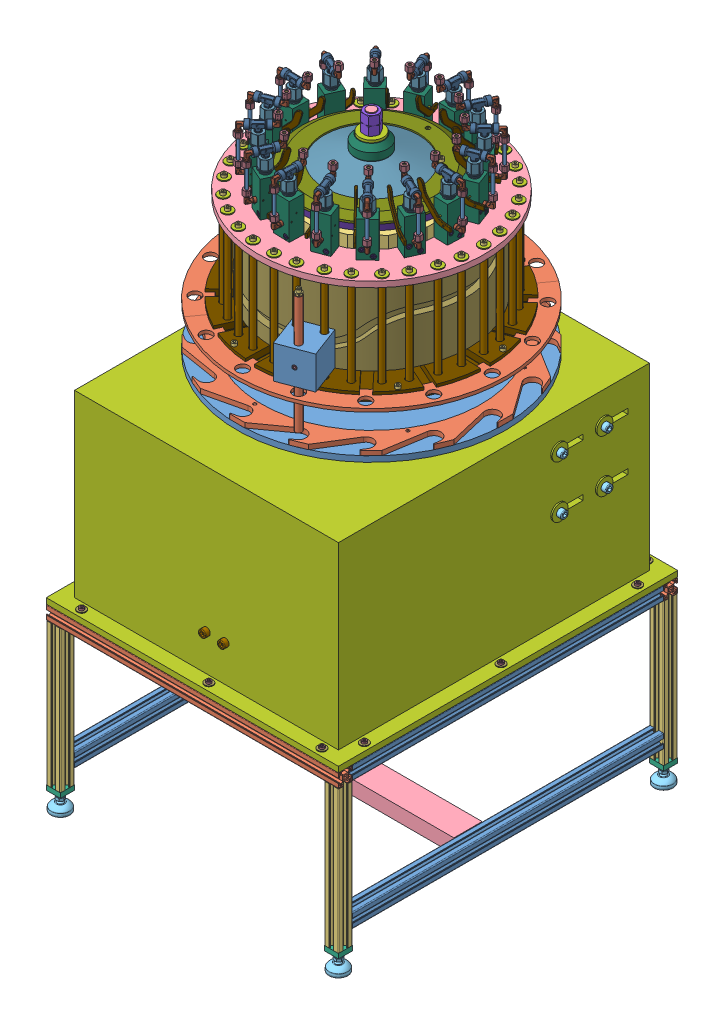
SolidWorks assembly Assieme_FINALE, configuration Default. Lengths in mm. (continued)
Components (placement in the parent): (continued)
- assieme parte rotante-2: assieme parte rotante [Default] at (-160.1634 623.9178 -718.4345) x (0 1 0) z (-0.527591 0 0.849499) size (749.63 778.63 778.63) (continued)
  - asta scorrimento carello-18: asta scorrimento carello [Default] at (287.5433 -61.3104 206.5173) x (0 -0.130526 -0.991445) z (-1 0 0) size (12 12 225)
  - asta scorrimento carello-19: asta scorrimento carello [Default] at (287.5433 -135.0285 252.8771) x (0 -0.5 -0.866025) z (-1 0 0) size (12 12 225)
  - asta scorrimento carello-20: asta scorrimento carello [Default] at (287.5433 -185.3939 323.9186) x (0 -0.793353 -0.608761) z (-1 0 0) size (12 12 225)
  - asta scorrimento carello-21: asta scorrimento carello [Default] at (287.5433 -204.7392 408.8264) x (0 -0.965926 -0.258819) z (-1 0 0) size (12 12 225)
  - asta scorrimento carello-22: asta scorrimento carello [Default] at (287.5433 -190.119 494.6741) x (0 -0.991445 0.130526) z (-1 0 0) size (12 12 225)
  - asta scorrimento carello-23: asta scorrimento carello [Default] at (287.5433 -143.7592 568.3922) x (0 -0.866025 0.5) z (-1 0 0) size (12 12 225)
  - asta scorrimento carello-24: asta scorrimento carello [Default] at (287.5433 -72.7177 618.7576) x (0 -0.608761 0.793353) z (-1 0 0) size (12 12 225)
  - asta scorrimento carello-25: asta scorrimento carello [Default] at (287.5433 12.1901 638.1029) x (0 -0.258819 0.965926) z (-1 0 0) size (12 12 225)
  - asta scorrimento carello-26: asta scorrimento carello [Default] at (287.5433 98.0378 623.4827) x (0 0.130526 0.991445) z (-1 0 0) size (12 12 225)
  - asta scorrimento carello-27: asta scorrimento carello [Default] at (287.5433 171.7559 577.1229) x (0 0.5 0.866025) z (-1 0 0) size (12 12 225)
  - asta scorrimento carello-28: asta scorrimento carello [Default] at (287.5433 222.1213 506.0814) x (0 0.793353 0.608761) z (-1 0 0) size (12 12 225)
  - asta scorrimento carello-29: asta scorrimento carello [Default] at (287.5433 241.4666 421.1736) x (0 0.965926 0.258819) z (-1 0 0) size (12 12 225)
  - asta scorrimento carello-30: asta scorrimento carello [Default] at (287.5433 226.8464 335.3259) x (0 0.991445 -0.130526) z (-1 0 0) size (12 12 225)
  - asta scorrimento carello-31: asta scorrimento carello [Default] at (287.5433 180.4866 261.6078) x (0 0.866025 -0.5) z (-1 0 0) size (12 12 225)
  - asta scorrimento carello-32: asta scorrimento carello [Default] at (287.5433 109.4451 211.2424) x (0 0.608761 -0.793353) z (-1 0 0) size (12 12 225)
  - rondella M6-129: rondella M6 [Washer ISO 7094 - 6] at (400.0433 -61.3104 206.5173) x (-1 0 0) z (0 0.991445 -0.130526) size (2 22 22)
  - rondella M6-130: rondella M6 [Washer ISO 7094 - 6] at (400.0433 -135.0285 252.8771) x (-1 0 0) z (0 0.866025 -0.5) size (2 22 22)
  - rondella M6-131: rondella M6 [Washer ISO 7094 - 6] at (400.0433 -185.3939 323.9186) x (-1 0 0) z (0 0.608761 -0.793353) size (2 22 22)
  - rondella M6-132: rondella M6 [Washer ISO 7094 - 6] at (400.0433 -204.7392 408.8264) x (-1 0 0) z (0 0.258819 -0.965926) size (2 22 22)
  - rondella M6-133: rondella M6 [Washer ISO 7094 - 6] at (400.0433 -190.119 494.6741) x (-1 0 0) z (0 -0.130526 -0.991445) size (2 22 22)
  - rondella M6-134: rondella M6 [Washer ISO 7094 - 6] at (400.0433 -143.7592 568.3922) x (-1 0 0) z (0 -0.5 -0.866025) size (2 22 22)
  - rondella M6-135: rondella M6 [Washer ISO 7094 - 6] at (400.0433 -72.7177 618.7576) x (-1 0 0) z (0 -0.793353 -0.608761) size (2 22 22)
  - rondella M6-136: rondella M6 [Washer ISO 7094 - 6] at (400.0433 12.1901 638.1029) x (-1 0 0) z (0 -0.965926 -0.258819) size (2 22 22)
  - rondella M6-137: rondella M6 [Washer ISO 7094 - 6] at (400.0433 98.0378 623.4827) x (-1 0 0) z (0 -0.991445 0.130526) size (2 22 22)
  - rondella M6-138: rondella M6 [Washer ISO 7094 - 6] at (400.0433 171.7559 577.1229) x (-1 0 0) z (0 -0.866025 0.5) size (2 22 22)
  - rondella M6-139: rondella M6 [Washer ISO 7094 - 6] at (400.0433 222.1213 506.0814) x (-1 0 0) z (0 -0.608761 0.793353) size (2 22 22)
  - rondella M6-140: rondella M6 [Washer ISO 7094 - 6] at (400.0433 241.4666 421.1736) x (-1 0 0) z (0 -0.258819 0.965926) size (2 22 22)
  - rondella M6-141: rondella M6 [Washer ISO 7094 - 6] at (400.0433 226.8464 335.3259) x (-1 0 0) z (0 0.130526 0.991445) size (2 22 22)
  - rondella M6-142: rondella M6 [Washer ISO 7094 - 6] at (400.0433 180.4866 261.6078) x (-1 0 0) z (0 0.5 0.866025) size (2 22 22)
  - rondella M6-143: rondella M6 [Washer ISO 7094 - 6] at (400.0433 109.4451 211.2424) x (-1 0 0) z (0 0.793353 0.608761) size (2 22 22)
  - M6 16mm-50: M6 16mm [ISO 4762 M6 x 16 - 16N] at (408.0433 -61.3104 206.5173) x (-1 0 0) z (0 0.130526 0.991445) size (22 10 10)
  - M6 16mm-51: M6 16mm [ISO 4762 M6 x 16 - 16N] at (408.0433 -135.0285 252.8771) x (-1 0 0) z (0 0.5 0.866025) size (22 10 10)
  - M6 16mm-52: M6 16mm [ISO 4762 M6 x 16 - 16N] at (408.0433 -185.3939 323.9186) x (-1 0 0) z (0 0.793353 0.608761) size (22 10 10)
  - M6 16mm-53: M6 16mm [ISO 4762 M6 x 16 - 16N] at (408.0433 -204.7392 408.8264) x (-1 0 0) z (0 0.965926 0.258819) size (22 10 10)
  - M6 16mm-54: M6 16mm [ISO 4762 M6 x 16 - 16N] at (408.0433 -190.119 494.6741) x (-1 0 0) z (0 0.991445 -0.130526) size (22 10 10)
  - M6 16mm-55: M6 16mm [ISO 4762 M6 x 16 - 16N] at (408.0433 -143.7592 568.3922) x (-1 0 0) z (0 0.866025 -0.5) size (22 10 10)
  - M6 16mm-56: M6 16mm [ISO 4762 M6 x 16 - 16N] at (408.0433 -72.7177 618.7576) x (-1 0 0) z (0 0.608761 -0.793353) size (22 10 10)
  - M6 16mm-57: M6 16mm [ISO 4762 M6 x 16 - 16N] at (408.0433 12.1901 638.1029) x (-1 0 0) z (0 0.258819 -0.965926) size (22 10 10)
  - M6 16mm-58: M6 16mm [ISO 4762 M6 x 16 - 16N] at (408.0433 98.0378 623.4827) x (-1 0 0) z (0 -0.130526 -0.991445) size (22 10 10)
  - M6 16mm-59: M6 16mm [ISO 4762 M6 x 16 - 16N] at (408.0433 171.7559 577.1229) x (-1 0 0) z (0 -0.5 -0.866025) size (22 10 10)
  - M6 16mm-60: M6 16mm [ISO 4762 M6 x 16 - 16N] at (408.0433 222.1213 506.0814) x (-1 0 0) z (0 -0.793353 -0.608761) size (22 10 10)
  - M6 16mm-61: M6 16mm [ISO 4762 M6 x 16 - 16N] at (408.0433 241.4666 421.1736) x (-1 0 0) z (0 -0.965926 -0.258819) size (22 10 10)
  - M6 16mm-62: M6 16mm [ISO 4762 M6 x 16 - 16N] at (408.0433 226.8464 335.3259) x (-1 0 0) z (0 -0.991445 0.130526) size (22 10 10)
  - M6 16mm-63: M6 16mm [ISO 4762 M6 x 16 - 16N] at (408.0433 180.4866 261.6078) x (-1 0 0) z (0 -0.866025 0.5) size (22 10 10)
  - M6 16mm-64: M6 16mm [ISO 4762 M6 x 16 - 16N] at (408.0433 109.4451 211.2424) x (-1 0 0) z (0 -0.608761 0.793353) size (22 10 10)
  - AssiemeValvola-2: AssiemeValvola [Default] at (515.3257 40.5532 246.4544) x (0 -0.130526 0.991445) z (0 0.991445 0.130526) size (90.26 138.63 38)
    - RaccordoT-1: RaccordoT [Default] at origin size (43 29.75 16.5)
    - Raccordo a L-1: Raccordo a L [Default] at (-30 0 0) x (0 -1 0) z (0 0 -1) size (28.34 25.51 14.01)
      - 1809_06_10_01-1: 1809_06_10_01 [Default] at origin size (22.49 23 10)
      - 1809_06_10_02-1: 1809_06_10_02 [Default] at origin size (6.5 8.5 8.5)
      - 1809_06_10_03-1: 1809_06_10_03 [Default] at origin size (11.02 15.01 14.01)
    - Raccordo a L-2: Raccordo a L [Default] at (30 0 0) x (0 1 0) z (0 0 -1) size (28.34 25.51 14.01)
      - 1809_06_10_01-1: 1809_06_10_01 [Default] at origin size (22.49 23 10)
      - 1809_06_10_02-1: 1809_06_10_02 [Default] at origin size (6.5 8.5 8.5)
      - 1809_06_10_03-1: 1809_06_10_03 [Default] at origin size (11.02 15.01 14.01)
    - TappoChiusura-1: TappoChiusura [Default] at (0 -32 0) x (0 -1 0) z (0 0 1) size (38.28 26.74 26.74)
    - CorpoValvola-1: CorpoValvola [Default] at (-15 -115.2824 0) size (30 75 34)
    - Raccordo a L-3: Raccordo a L [Default] at (-30 -88.2824 0) x (0 1 0) z (0 0 1) size (28.34 25.51 14.01)
      - 1809_06_10_01-1: 1809_06_10_01 [Default] at origin size (22.49 23 10)
      - 1809_06_10_02-1: 1809_06_10_02 [Default] at origin size (6.5 8.5 8.5)
      - 1809_06_10_03-1: 1809_06_10_03 [Default] at origin size (11.02 15.01 14.01)
    - Spina_3x38-1: Spina_3x38 [Default] at (0 -68.2824 -21) x (-1 0 0) z (0 0 1) size (3 3 38)
    - Spina_3x38-2: Spina_3x38 [Default] at (-10 -80.2824 -21) x (0.996193 0.087174 0) z (0 0 1) size (3 3 38)
    - M5 40mm-3: M5 40mm [ISO 4762 M5 x 40 - 40N] at (-14.6 -108.7824 9) size (45 8.5 8.5)
    - M5 40mm-2: M5 40mm [ISO 4762 M5 x 40 - 40N] at (-14.6 -96.7824 -9) size (45 8.5 8.5)
    - LevaValvola-1: LevaValvola [Default] at (-24.507 -86.571 -17) x (0.996193 0.087174 0) z (0 0 1) size (77.55 60.2 4)
    - Tubo-1: Tubo [Default] at (-30 -15.9665 0) x (1 0 0) z (0 -1 0) size (6 6 56.4)
  - AssiemeValvola-3: AssiemeValvola [Default] at (515.3257 -25.6355 250.7926) x (0 0.258819 0.965926) z (0 0.965926 -0.258819) size (90.26 138.63 38)
    - RaccordoT-1: RaccordoT [Default] at origin size (43 29.75 16.5)
    - Raccordo a L-1: Raccordo a L [Default] at (-30 0 0) x (0 -1 0) z (0 0 -1) size (28.34 25.51 14.01)
      - 1809_06_10_01-1: 1809_06_10_01 [Default] at origin size (22.49 23 10)
      - 1809_06_10_02-1: 1809_06_10_02 [Default] at origin size (6.5 8.5 8.5)
      - 1809_06_10_03-1: 1809_06_10_03 [Default] at origin size (11.02 15.01 14.01)
    - Raccordo a L-2: Raccordo a L [Default] at (30 0 0) x (0 1 0) z (0 0 -1) size (28.34 25.51 14.01)
      - 1809_06_10_01-1: 1809_06_10_01 [Default] at origin size (22.49 23 10)
      - 1809_06_10_02-1: 1809_06_10_02 [Default] at origin size (6.5 8.5 8.5)
      - 1809_06_10_03-1: 1809_06_10_03 [Default] at origin size (11.02 15.01 14.01)
    - TappoChiusura-1: TappoChiusura [Default] at (0 -32 0) x (0 -1 0) z (0 0 1) size (38.28 26.74 26.74)
    - CorpoValvola-1: CorpoValvola [Default] at (-15 -115.2824 0) size (30 75 34)
    - Raccordo a L-3: Raccordo a L [Default] at (-30 -88.2824 0) x (0 1 0) z (0 0 1) size (28.34 25.51 14.01)
      - 1809_06_10_01-1: 1809_06_10_01 [Default] at origin size (22.49 23 10)
      - 1809_06_10_02-1: 1809_06_10_02 [Default] at origin size (6.5 8.5 8.5)
      - 1809_06_10_03-1: 1809_06_10_03 [Default] at origin size (11.02 15.01 14.01)
    - Spina_3x38-1: Spina_3x38 [Default] at (0 -68.2824 -21) x (-1 0 0) z (0 0 1) size (3 3 38)
    - Spina_3x38-2: Spina_3x38 [Default] at (-10 -80.2824 -21) x (0.996193 0.087174 0) z (0 0 1) size (3 3 38)
    - M5 40mm-3: M5 40mm [ISO 4762 M5 x 40 - 40N] at (-14.6 -108.7824 9) size (45 8.5 8.5)
    - M5 40mm-2: M5 40mm [ISO 4762 M5 x 40 - 40N] at (-14.6 -96.7824 -9) size (45 8.5 8.5)
    - LevaValvola-1: LevaValvola [Default] at (-24.507 -86.571 -17) x (0.996193 0.087174 0) z (0 0 1) size (77.55 60.2 4)
    - Tubo-1: Tubo [Default] at (-30 -15.9665 0) x (1 0 0) z (0 -1 0) size (6 6 56.4)
  - AssiemeValvola-4: AssiemeValvola [Default] at (515.3257 -85.1257 280.1299) x (0 0.608761 0.793353) z (0 0.793353 -0.608761) size (90.26 138.63 38)
    - RaccordoT-1: RaccordoT [Default] at origin size (43 29.75 16.5)
    - Raccordo a L-1: Raccordo a L [Default] at (-30 0 0) x (0 -1 0) z (0 0 -1) size (28.34 25.51 14.01)
      - 1809_06_10_01-1: 1809_06_10_01 [Default] at origin size (22.49 23 10)
      - 1809_06_10_02-1: 1809_06_10_02 [Default] at origin size (6.5 8.5 8.5)
      - 1809_06_10_03-1: 1809_06_10_03 [Default] at origin size (11.02 15.01 14.01)
    - Raccordo a L-2: Raccordo a L [Default] at (30 0 0) x (0 1 0) z (0 0 -1) size (28.34 25.51 14.01)
      - 1809_06_10_01-1: 1809_06_10_01 [Default] at origin size (22.49 23 10)
      - 1809_06_10_02-1: 1809_06_10_02 [Default] at origin size (6.5 8.5 8.5)
      - 1809_06_10_03-1: 1809_06_10_03 [Default] at origin size (11.02 15.01 14.01)
    - TappoChiusura-1: TappoChiusura [Default] at (0 -32 0) x (0 -1 0) z (0 0 1) size (38.28 26.74 26.74)
    - CorpoValvola-1: CorpoValvola [Default] at (-15 -115.2824 0) size (30 75 34)
    - Raccordo a L-3: Raccordo a L [Default] at (-30 -88.2824 0) x (0 1 0) z (0 0 1) size (28.34 25.51 14.01)
      - 1809_06_10_01-1: 1809_06_10_01 [Default] at origin size (22.49 23 10)
      - 1809_06_10_02-1: 1809_06_10_02 [Default] at origin size (6.5 8.5 8.5)
      - 1809_06_10_03-1: 1809_06_10_03 [Default] at origin size (11.02 15.01 14.01)
    - Spina_3x38-1: Spina_3x38 [Default] at (0 -68.2824 -21) x (-1 0 0) z (0 0 1) size (3 3 38)
    - Spina_3x38-2: Spina_3x38 [Default] at (-10 -80.2824 -21) x (0.996193 0.087174 0) z (0 0 1) size (3 3 38)
    - M5 40mm-3: M5 40mm [ISO 4762 M5 x 40 - 40N] at (-14.6 -108.7824 9) size (45 8.5 8.5)
    - M5 40mm-2: M5 40mm [ISO 4762 M5 x 40 - 40N] at (-14.6 -96.7824 -9) size (45 8.5 8.5)
    - LevaValvola-1: LevaValvola [Default] at (-24.507 -86.571 -17) x (0.996193 0.087174 0) z (0 0 1) size (77.55 60.2 4)
    - Tubo-1: Tubo [Default] at (-30 -15.9665 0) x (1 0 0) z (0 -1 0) size (6 6 56.4)
  - AssiemeValvola-5: AssiemeValvola [Default] at (515.3257 -128.8606 330) x (0 0.866025 0.5) z (0 0.5 -0.866025) size (90.26 138.63 38)
    - RaccordoT-1: RaccordoT [Default] at origin size (43 29.75 16.5)
    - Raccordo a L-1: Raccordo a L [Default] at (-30 0 0) x (0 -1 0) z (0 0 -1) size (28.34 25.51 14.01)
      - 1809_06_10_01-1: 1809_06_10_01 [Default] at origin size (22.49 23 10)
      - 1809_06_10_02-1: 1809_06_10_02 [Default] at origin size (6.5 8.5 8.5)
      - 1809_06_10_03-1: 1809_06_10_03 [Default] at origin size (11.02 15.01 14.01)
    - Raccordo a L-2: Raccordo a L [Default] at (30 0 0) x (0 1 0) z (0 0 -1) size (28.34 25.51 14.01)
      - 1809_06_10_01-1: 1809_06_10_01 [Default] at origin size (22.49 23 10)
      - 1809_06_10_02-1: 1809_06_10_02 [Default] at origin size (6.5 8.5 8.5)
      - 1809_06_10_03-1: 1809_06_10_03 [Default] at origin size (11.02 15.01 14.01)
    - TappoChiusura-1: TappoChiusura [Default] at (0 -32 0) x (0 -1 0) z (0 0 1) size (38.28 26.74 26.74)
    - CorpoValvola-1: CorpoValvola [Default] at (-15 -115.2824 0) size (30 75 34)
    - Raccordo a L-3: Raccordo a L [Default] at (-30 -88.2824 0) x (0 1 0) z (0 0 1) size (28.34 25.51 14.01)
      - 1809_06_10_01-1: 1809_06_10_01 [Default] at origin size (22.49 23 10)
      - 1809_06_10_02-1: 1809_06_10_02 [Default] at origin size (6.5 8.5 8.5)
      - 1809_06_10_03-1: 1809_06_10_03 [Default] at origin size (11.02 15.01 14.01)
    - Spina_3x38-1: Spina_3x38 [Default] at (0 -68.2824 -21) x (-1 0 0) z (0 0 1) size (3 3 38)
    - Spina_3x38-2: Spina_3x38 [Default] at (-10 -80.2824 -21) x (0.996193 0.087174 0) z (0 0 1) size (3 3 38)
    - M5 40mm-3: M5 40mm [ISO 4762 M5 x 40 - 40N] at (-14.6 -108.7824 9) size (45 8.5 8.5)
    - M5 40mm-2: M5 40mm [ISO 4762 M5 x 40 - 40N] at (-14.6 -96.7824 -9) size (45 8.5 8.5)
    - LevaValvola-1: LevaValvola [Default] at (-24.507 -86.571 -17) x (0.996193 0.087174 0) z (0 0 1) size (77.55 60.2 4)
    - Tubo-1: Tubo [Default] at (-30 -15.9665 0) x (1 0 0) z (0 -1 0) size (6 6 56.4)
  - AssiemeValvola-6: AssiemeValvola [Default] at (515.3257 -150.1819 392.8105) x (0 0.991445 0.130526) z (0 0.130526 -0.991445) size (90.26 138.63 38)
    - RaccordoT-1: RaccordoT [Default] at origin size (43 29.75 16.5)
    - Raccordo a L-1: Raccordo a L [Default] at (-30 0 0) x (0 -1 0) z (0 0 -1) size (28.34 25.51 14.01)
      - 1809_06_10_01-1: 1809_06_10_01 [Default] at origin size (22.49 23 10)
      - 1809_06_10_02-1: 1809_06_10_02 [Default] at origin size (6.5 8.5 8.5)
      - 1809_06_10_03-1: 1809_06_10_03 [Default] at origin size (11.02 15.01 14.01)
    - Raccordo a L-2: Raccordo a L [Default] at (30 0 0) x (0 1 0) z (0 0 -1) size (28.34 25.51 14.01)
      - 1809_06_10_01-1: 1809_06_10_01 [Default] at origin size (22.49 23 10)
      - 1809_06_10_02-1: 1809_06_10_02 [Default] at origin size (6.5 8.5 8.5)
      - 1809_06_10_03-1: 1809_06_10_03 [Default] at origin size (11.02 15.01 14.01)
    - TappoChiusura-1: TappoChiusura [Default] at (0 -32 0) x (0 -1 0) z (0 0 1) size (38.28 26.74 26.74)
    - CorpoValvola-1: CorpoValvola [Default] at (-15 -115.2824 0) size (30 75 34)
    - Raccordo a L-3: Raccordo a L [Default] at (-30 -88.2824 0) x (0 1 0) z (0 0 1) size (28.34 25.51 14.01)
      - 1809_06_10_01-1: 1809_06_10_01 [Default] at origin size (22.49 23 10)
      - 1809_06_10_02-1: 1809_06_10_02 [Default] at origin size (6.5 8.5 8.5)
      - 1809_06_10_03-1: 1809_06_10_03 [Default] at origin size (11.02 15.01 14.01)
    - Spina_3x38-1: Spina_3x38 [Default] at (0 -68.2824 -21) x (-1 0 0) z (0 0 1) size (3 3 38)
    - Spina_3x38-2: Spina_3x38 [Default] at (-10 -80.2824 -21) x (0.996193 0.087174 0) z (0 0 1) size (3 3 38)
    - M5 40mm-3: M5 40mm [ISO 4762 M5 x 40 - 40N] at (-14.6 -108.7824 9) size (45 8.5 8.5)
    - M5 40mm-2: M5 40mm [ISO 4762 M5 x 40 - 40N] at (-14.6 -96.7824 -9) size (45 8.5 8.5)
    - LevaValvola-1: LevaValvola [Default] at (-24.507 -86.571 -17) x (0.996193 0.087174 0) z (0 0 1) size (77.55 60.2 4)
    - Tubo-1: Tubo [Default] at (-30 -15.9665 0) x (1 0 0) z (0 -1 0) size (6 6 56.4)
  - AssiemeValvola-7: AssiemeValvola [Default] at (515.3257 -145.8437 458.9992) x (0 0.965926 -0.258819) z (0 -0.258819 -0.965926) size (90.26 138.63 38)
    - RaccordoT-1: RaccordoT [Default] at origin size (43 29.75 16.5)
    - Raccordo a L-1: Raccordo a L [Default] at (-30 0 0) x (0 -1 0) z (0 0 -1) size (28.34 25.51 14.01)
      - 1809_06_10_01-1: 1809_06_10_01 [Default] at origin size (22.49 23 10)
      - 1809_06_10_02-1: 1809_06_10_02 [Default] at origin size (6.5 8.5 8.5)
      - 1809_06_10_03-1: 1809_06_10_03 [Default] at origin size (11.02 15.01 14.01)
    - Raccordo a L-2: Raccordo a L [Default] at (30 0 0) x (0 1 0) z (0 0 -1) size (28.34 25.51 14.01)
      - 1809_06_10_01-1: 1809_06_10_01 [Default] at origin size (22.49 23 10)
      - 1809_06_10_02-1: 1809_06_10_02 [Default] at origin size (6.5 8.5 8.5)
      - 1809_06_10_03-1: 1809_06_10_03 [Default] at origin size (11.02 15.01 14.01)
    - TappoChiusura-1: TappoChiusura [Default] at (0 -32 0) x (0 -1 0) z (0 0 1) size (38.28 26.74 26.74)
    - CorpoValvola-1: CorpoValvola [Default] at (-15 -115.2824 0) size (30 75 34)
    - Raccordo a L-3: Raccordo a L [Default] at (-30 -88.2824 0) x (0 1 0) z (0 0 1) size (28.34 25.51 14.01)
      - 1809_06_10_01-1: 1809_06_10_01 [Default] at origin size (22.49 23 10)
      - 1809_06_10_02-1: 1809_06_10_02 [Default] at origin size (6.5 8.5 8.5)
      - 1809_06_10_03-1: 1809_06_10_03 [Default] at origin size (11.02 15.01 14.01)
    - Spina_3x38-1: Spina_3x38 [Default] at (0 -68.2824 -21) x (-1 0 0) z (0 0 1) size (3 3 38)
    - Spina_3x38-2: Spina_3x38 [Default] at (-10 -80.2824 -21) x (0.996193 0.087174 0) z (0 0 1) size (3 3 38)
    - M5 40mm-3: M5 40mm [ISO 4762 M5 x 40 - 40N] at (-14.6 -108.7824 9) size (45 8.5 8.5)
    - M5 40mm-2: M5 40mm [ISO 4762 M5 x 40 - 40N] at (-14.6 -96.7824 -9) size (45 8.5 8.5)
    - LevaValvola-1: LevaValvola [Default] at (-24.507 -86.571 -17) x (0.996193 0.087174 0) z (0 0 1) size (77.55 60.2 4)
    - Tubo-1: Tubo [Default] at (-30 -15.9665 0) x (1 0 0) z (0 -1 0) size (6 6 56.4)
  - AssiemeValvola-8: AssiemeValvola [Default] at (515.3257 -116.5064 518.4894) x (0 0.793353 -0.608761) z (0 -0.608761 -0.793353) size (90.26 138.63 38)
    - RaccordoT-1: RaccordoT [Default] at origin size (43 29.75 16.5)
    - Raccordo a L-1: Raccordo a L [Default] at (-30 0 0) x (0 -1 0) z (0 0 -1) size (28.34 25.51 14.01)
      - 1809_06_10_01-1: 1809_06_10_01 [Default] at origin size (22.49 23 10)
      - 1809_06_10_02-1: 1809_06_10_02 [Default] at origin size (6.5 8.5 8.5)
      - 1809_06_10_03-1: 1809_06_10_03 [Default] at origin size (11.02 15.01 14.01)
    - Raccordo a L-2: Raccordo a L [Default] at (30 0 0) x (0 1 0) z (0 0 -1) size (28.34 25.51 14.01)
      - 1809_06_10_01-1: 1809_06_10_01 [Default] at origin size (22.49 23 10)
      - 1809_06_10_02-1: 1809_06_10_02 [Default] at origin size (6.5 8.5 8.5)
      - 1809_06_10_03-1: 1809_06_10_03 [Default] at origin size (11.02 15.01 14.01)
    - TappoChiusura-1: TappoChiusura [Default] at (0 -32 0) x (0 -1 0) z (0 0 1) size (38.28 26.74 26.74)
    - CorpoValvola-1: CorpoValvola [Default] at (-15 -115.2824 0) size (30 75 34)
    - Raccordo a L-3: Raccordo a L [Default] at (-30 -88.2824 0) x (0 1 0) z (0 0 1) size (28.34 25.51 14.01)
      - 1809_06_10_01-1: 1809_06_10_01 [Default] at origin size (22.49 23 10)
      - 1809_06_10_02-1: 1809_06_10_02 [Default] at origin size (6.5 8.5 8.5)
      - 1809_06_10_03-1: 1809_06_10_03 [Default] at origin size (11.02 15.01 14.01)
    - Spina_3x38-1: Spina_3x38 [Default] at (0 -68.2824 -21) x (-1 0 0) z (0 0 1) size (3 3 38)
    - Spina_3x38-2: Spina_3x38 [Default] at (-10 -80.2824 -21) x (0.996193 0.087174 0) z (0 0 1) size (3 3 38)
    - M5 40mm-3: M5 40mm [ISO 4762 M5 x 40 - 40N] at (-14.6 -108.7824 9) size (45 8.5 8.5)
    - M5 40mm-2: M5 40mm [ISO 4762 M5 x 40 - 40N] at (-14.6 -96.7824 -9) size (45 8.5 8.5)
    - LevaValvola-1: LevaValvola [Default] at (-24.507 -86.571 -17) x (0.996193 0.087174 0) z (0 0 1) size (77.55 60.2 4)
    - Tubo-1: Tubo [Default] at (-30 -15.9665 0) x (1 0 0) z (0 -1 0) size (6 6 56.4)
  - AssiemeValvola-9: AssiemeValvola [Default] at (515.3257 -66.6363 562.2243) x (0 0.5 -0.866025) z (0 -0.866025 -0.5) size (90.26 138.63 38)
    - RaccordoT-1: RaccordoT [Default] at origin size (43 29.75 16.5)
    - Raccordo a L-1: Raccordo a L [Default] at (-30 0 0) x (0 -1 0) z (0 0 -1) size (28.34 25.51 14.01)
      - 1809_06_10_01-1: 1809_06_10_01 [Default] at origin size (22.49 23 10)
      - 1809_06_10_02-1: 1809_06_10_02 [Default] at origin size (6.5 8.5 8.5)
      - 1809_06_10_03-1: 1809_06_10_03 [Default] at origin size (11.02 15.01 14.01)
    - Raccordo a L-2: Raccordo a L [Default] at (30 0 0) x (0 1 0) z (0 0 -1) size (28.34 25.51 14.01)
      - 1809_06_10_01-1: 1809_06_10_01 [Default] at origin size (22.49 23 10)
      - 1809_06_10_02-1: 1809_06_10_02 [Default] at origin size (6.5 8.5 8.5)
      - 1809_06_10_03-1: 1809_06_10_03 [Default] at origin size (11.02 15.01 14.01)
    - TappoChiusura-1: TappoChiusura [Default] at (0 -32 0) x (0 -1 0) z (0 0 1) size (38.28 26.74 26.74)
    - CorpoValvola-1: CorpoValvola [Default] at (-15 -115.2824 0) size (30 75 34)
    - Raccordo a L-3: Raccordo a L [Default] at (-30 -88.2824 0) x (0 1 0) z (0 0 1) size (28.34 25.51 14.01)
      - 1809_06_10_01-1: 1809_06_10_01 [Default] at origin size (22.49 23 10)
      - 1809_06_10_02-1: 1809_06_10_02 [Default] at origin size (6.5 8.5 8.5)
      - 1809_06_10_03-1: 1809_06_10_03 [Default] at origin size (11.02 15.01 14.01)
    - Spina_3x38-1: Spina_3x38 [Default] at (0 -68.2824 -21) x (-1 0 0) z (0 0 1) size (3 3 38)
    - Spina_3x38-2: Spina_3x38 [Default] at (-10 -80.2824 -21) x (0.996193 0.087174 0) z (0 0 1) size (3 3 38)
    - M5 40mm-3: M5 40mm [ISO 4762 M5 x 40 - 40N] at (-14.6 -108.7824 9) size (45 8.5 8.5)
    - M5 40mm-2: M5 40mm [ISO 4762 M5 x 40 - 40N] at (-14.6 -96.7824 -9) size (45 8.5 8.5)
    - LevaValvola-1: LevaValvola [Default] at (-24.507 -86.571 -17) x (0.996193 0.087174 0) z (0 0 1) size (77.55 60.2 4)
    - Tubo-1: Tubo [Default] at (-30 -15.9665 0) x (1 0 0) z (0 -1 0) size (6 6 56.4)
  - AssiemeValvola-10: AssiemeValvola [Default] at (515.3257 -3.8258 583.5456) x (0 0.130526 -0.991445) z (0 -0.991445 -0.130526) size (90.26 138.63 38)
    - RaccordoT-1: RaccordoT [Default] at origin size (43 29.75 16.5)
    - Raccordo a L-1: Raccordo a L [Default] at (-30 0 0) x (0 -1 0) z (0 0 -1) size (28.34 25.51 14.01)
      - 1809_06_10_01-1: 1809_06_10_01 [Default] at origin size (22.49 23 10)
      - 1809_06_10_02-1: 1809_06_10_02 [Default] at origin size (6.5 8.5 8.5)
      - 1809_06_10_03-1: 1809_06_10_03 [Default] at origin size (11.02 15.01 14.01)
    - Raccordo a L-2: Raccordo a L [Default] at (30 0 0) x (0 1 0) z (0 0 -1) size (28.34 25.51 14.01)
      - 1809_06_10_01-1: 1809_06_10_01 [Default] at origin size (22.49 23 10)
      - 1809_06_10_02-1: 1809_06_10_02 [Default] at origin size (6.5 8.5 8.5)
      - 1809_06_10_03-1: 1809_06_10_03 [Default] at origin size (11.02 15.01 14.01)
    - TappoChiusura-1: TappoChiusura [Default] at (0 -32 0) x (0 -1 0) z (0 0 1) size (38.28 26.74 26.74)
    - CorpoValvola-1: CorpoValvola [Default] at (-15 -115.2824 0) size (30 75 34)
    - Raccordo a L-3: Raccordo a L [Default] at (-30 -88.2824 0) x (0 1 0) z (0 0 1) size (28.34 25.51 14.01)
      - 1809_06_10_01-1: 1809_06_10_01 [Default] at origin size (22.49 23 10)
      - 1809_06_10_02-1: 1809_06_10_02 [Default] at origin size (6.5 8.5 8.5)
      - 1809_06_10_03-1: 1809_06_10_03 [Default] at origin size (11.02 15.01 14.01)
    - Spina_3x38-1: Spina_3x38 [Default] at (0 -68.2824 -21) x (-1 0 0) z (0 0 1) size (3 3 38)
    - Spina_3x38-2: Spina_3x38 [Default] at (-10 -80.2824 -21) x (0.996193 0.087174 0) z (0 0 1) size (3 3 38)
    - M5 40mm-3: M5 40mm [ISO 4762 M5 x 40 - 40N] at (-14.6 -108.7824 9) size (45 8.5 8.5)
    - M5 40mm-2: M5 40mm [ISO 4762 M5 x 40 - 40N] at (-14.6 -96.7824 -9) size (45 8.5 8.5)
    - LevaValvola-1: LevaValvola [Default] at (-24.507 -86.571 -17) x (0.996193 0.087174 0) z (0 0 1) size (77.55 60.2 4)
    - Tubo-1: Tubo [Default] at (-30 -15.9665 0) x (1 0 0) z (0 -1 0) size (6 6 56.4)
  - AssiemeValvola-11: AssiemeValvola [Default] at (515.3257 62.3629 579.2074) x (0 -0.258819 -0.965926) z (0 -0.965926 0.258819) size (90.26 138.63 38)
    - RaccordoT-1: RaccordoT [Default] at origin size (43 29.75 16.5)
    - Raccordo a L-1: Raccordo a L [Default] at (-30 0 0) x (0 -1 0) z (0 0 -1) size (28.34 25.51 14.01)
      - 1809_06_10_01-1: 1809_06_10_01 [Default] at origin size (22.49 23 10)
      - 1809_06_10_02-1: 1809_06_10_02 [Default] at origin size (6.5 8.5 8.5)
      - 1809_06_10_03-1: 1809_06_10_03 [Default] at origin size (11.02 15.01 14.01)
    - Raccordo a L-2: Raccordo a L [Default] at (30 0 0) x (0 1 0) z (0 0 -1) size (28.34 25.51 14.01)
      - 1809_06_10_01-1: 1809_06_10_01 [Default] at origin size (22.49 23 10)
      - 1809_06_10_02-1: 1809_06_10_02 [Default] at origin size (6.5 8.5 8.5)
      - 1809_06_10_03-1: 1809_06_10_03 [Default] at origin size (11.02 15.01 14.01)
    - TappoChiusura-1: TappoChiusura [Default] at (0 -32 0) x (0 -1 0) z (0 0 1) size (38.28 26.74 26.74)
    - CorpoValvola-1: CorpoValvola [Default] at (-15 -115.2824 0) size (30 75 34)
    - Raccordo a L-3: Raccordo a L [Default] at (-30 -88.2824 0) x (0 1 0) z (0 0 1) size (28.34 25.51 14.01)
      - 1809_06_10_01-1: 1809_06_10_01 [Default] at origin size (22.49 23 10)
      - 1809_06_10_02-1: 1809_06_10_02 [Default] at origin size (6.5 8.5 8.5)
      - 1809_06_10_03-1: 1809_06_10_03 [Default] at origin size (11.02 15.01 14.01)
    - Spina_3x38-1: Spina_3x38 [Default] at (0 -68.2824 -21) x (-1 0 0) z (0 0 1) size (3 3 38)
    - Spina_3x38-2: Spina_3x38 [Default] at (-10 -80.2824 -21) x (0.996193 0.087174 0) z (0 0 1) size (3 3 38)
    - M5 40mm-3: M5 40mm [ISO 4762 M5 x 40 - 40N] at (-14.6 -108.7824 9) size (45 8.5 8.5)
    - M5 40mm-2: M5 40mm [ISO 4762 M5 x 40 - 40N] at (-14.6 -96.7824 -9) size (45 8.5 8.5)
    - LevaValvola-1: LevaValvola [Default] at (-24.507 -86.571 -17) x (0.996193 0.087174 0) z (0 0 1) size (77.55 60.2 4)
    - Tubo-1: Tubo [Default] at (-30 -15.9665 0) x (1 0 0) z (0 -1 0) size (6 6 56.4)
  - AssiemeValvola-12: AssiemeValvola [Default] at (515.3257 121.8531 549.8701) x (0 -0.608761 -0.793353) z (0 -0.793353 0.608761) size (90.26 138.63 38)
    - RaccordoT-1: RaccordoT [Default] at origin size (43 29.75 16.5)
    - Raccordo a L-1: Raccordo a L [Default] at (-30 0 0) x (0 -1 0) z (0 0 -1) size (28.34 25.51 14.01)
      - 1809_06_10_01-1: 1809_06_10_01 [Default] at origin size (22.49 23 10)
      - 1809_06_10_02-1: 1809_06_10_02 [Default] at origin size (6.5 8.5 8.5)
      - 1809_06_10_03-1: 1809_06_10_03 [Default] at origin size (11.02 15.01 14.01)
    - Raccordo a L-2: Raccordo a L [Default] at (30 0 0) x (0 1 0) z (0 0 -1) size (28.34 25.51 14.01)
      - 1809_06_10_01-1: 1809_06_10_01 [Default] at origin size (22.49 23 10)
      - 1809_06_10_02-1: 1809_06_10_02 [Default] at origin size (6.5 8.5 8.5)
      - 1809_06_10_03-1: 1809_06_10_03 [Default] at origin size (11.02 15.01 14.01)
    - TappoChiusura-1: TappoChiusura [Default] at (0 -32 0) x (0 -1 0) z (0 0 1) size (38.28 26.74 26.74)
    - CorpoValvola-1: CorpoValvola [Default] at (-15 -115.2824 0) size (30 75 34)
    - Raccordo a L-3: Raccordo a L [Default] at (-30 -88.2824 0) x (0 1 0) z (0 0 1) size (28.34 25.51 14.01)
      - 1809_06_10_01-1: 1809_06_10_01 [Default] at origin size (22.49 23 10)
      - 1809_06_10_02-1: 1809_06_10_02 [Default] at origin size (6.5 8.5 8.5)
      - 1809_06_10_03-1: 1809_06_10_03 [Default] at origin size (11.02 15.01 14.01)
    - Spina_3x38-1: Spina_3x38 [Default] at (0 -68.2824 -21) x (-1 0 0) z (0 0 1) size (3 3 38)
    - Spina_3x38-2: Spina_3x38 [Default] at (-10 -80.2824 -21) x (0.996193 0.087174 0) z (0 0 1) size (3 3 38)
    - M5 40mm-3: M5 40mm [ISO 4762 M5 x 40 - 40N] at (-14.6 -108.7824 9) size (45 8.5 8.5)
    - M5 40mm-2: M5 40mm [ISO 4762 M5 x 40 - 40N] at (-14.6 -96.7824 -9) size (45 8.5 8.5)
    - LevaValvola-1: LevaValvola [Default] at (-24.507 -86.571 -17) x (0.996193 0.087174 0) z (0 0 1) size (77.55 60.2 4)
    - Tubo-1: Tubo [Default] at (-30 -15.9665 0) x (1 0 0) z (0 -1 0) size (6 6 56.4)
  - AssiemeValvola-13: AssiemeValvola [Default] at (515.3257 165.588 500) x (0 -0.866025 -0.5) z (0 -0.5 0.866025) size (90.26 138.63 38)
    - RaccordoT-1: RaccordoT [Default] at origin size (43 29.75 16.5)
    - Raccordo a L-1: Raccordo a L [Default] at (-30 0 0) x (0 -1 0) z (0 0 -1) size (28.34 25.51 14.01)
      - 1809_06_10_01-1: 1809_06_10_01 [Default] at origin size (22.49 23 10)
      - 1809_06_10_02-1: 1809_06_10_02 [Default] at origin size (6.5 8.5 8.5)
      - 1809_06_10_03-1: 1809_06_10_03 [Default] at origin size (11.02 15.01 14.01)
    - Raccordo a L-2: Raccordo a L [Default] at (30 0 0) x (0 1 0) z (0 0 -1) size (28.34 25.51 14.01)
      - 1809_06_10_01-1: 1809_06_10_01 [Default] at origin size (22.49 23 10)
      - 1809_06_10_02-1: 1809_06_10_02 [Default] at origin size (6.5 8.5 8.5)
      - 1809_06_10_03-1: 1809_06_10_03 [Default] at origin size (11.02 15.01 14.01)
    - TappoChiusura-1: TappoChiusura [Default] at (0 -32 0) x (0 -1 0) z (0 0 1) size (38.28 26.74 26.74)
    - CorpoValvola-1: CorpoValvola [Default] at (-15 -115.2824 0) size (30 75 34)
    - Raccordo a L-3: Raccordo a L [Default] at (-30 -88.2824 0) x (0 1 0) z (0 0 1) size (28.34 25.51 14.01)
      - 1809_06_10_01-1: 1809_06_10_01 [Default] at origin size (22.49 23 10)
      - 1809_06_10_02-1: 1809_06_10_02 [Default] at origin size (6.5 8.5 8.5)
      - 1809_06_10_03-1: 1809_06_10_03 [Default] at origin size (11.02 15.01 14.01)
    - Spina_3x38-1: Spina_3x38 [Default] at (0 -68.2824 -21) x (-1 0 0) z (0 0 1) size (3 3 38)
    - Spina_3x38-2: Spina_3x38 [Default] at (-10 -80.2824 -21) x (0.996193 0.087174 0) z (0 0 1) size (3 3 38)
    - M5 40mm-3: M5 40mm [ISO 4762 M5 x 40 - 40N] at (-14.6 -108.7824 9) size (45 8.5 8.5)
    - M5 40mm-2: M5 40mm [ISO 4762 M5 x 40 - 40N] at (-14.6 -96.7824 -9) size (45 8.5 8.5)
    - LevaValvola-1: LevaValvola [Default] at (-24.507 -86.571 -17) x (0.996193 0.087174 0) z (0 0 1) size (77.55 60.2 4)
    - Tubo-1: Tubo [Default] at (-30 -15.9665 0) x (1 0 0) z (0 -1 0) size (6 6 56.4)
  - AssiemeValvola-14: AssiemeValvola [Default] at (515.3257 186.9093 437.1895) x (0 -0.991445 -0.130526) z (0 -0.130526 0.991445) size (90.26 138.63 38)
    - RaccordoT-1: RaccordoT [Default] at origin size (43 29.75 16.5)
    - Raccordo a L-1: Raccordo a L [Default] at (-30 0 0) x (0 -1 0) z (0 0 -1) size (28.34 25.51 14.01)
      - 1809_06_10_01-1: 1809_06_10_01 [Default] at origin size (22.49 23 10)
      - 1809_06_10_02-1: 1809_06_10_02 [Default] at origin size (6.5 8.5 8.5)
      - 1809_06_10_03-1: 1809_06_10_03 [Default] at origin size (11.02 15.01 14.01)
    - Raccordo a L-2: Raccordo a L [Default] at (30 0 0) x (0 1 0) z (0 0 -1) size (28.34 25.51 14.01)
      - 1809_06_10_01-1: 1809_06_10_01 [Default] at origin size (22.49 23 10)
      - 1809_06_10_02-1: 1809_06_10_02 [Default] at origin size (6.5 8.5 8.5)
      - 1809_06_10_03-1: 1809_06_10_03 [Default] at origin size (11.02 15.01 14.01)
    - TappoChiusura-1: TappoChiusura [Default] at (0 -32 0) x (0 -1 0) z (0 0 1) size (38.28 26.74 26.74)
    - CorpoValvola-1: CorpoValvola [Default] at (-15 -115.2824 0) size (30 75 34)
    - Raccordo a L-3: Raccordo a L [Default] at (-30 -88.2824 0) x (0 1 0) z (0 0 1) size (28.34 25.51 14.01)
      - 1809_06_10_01-1: 1809_06_10_01 [Default] at origin size (22.49 23 10)
      - 1809_06_10_02-1: 1809_06_10_02 [Default] at origin size (6.5 8.5 8.5)
      - 1809_06_10_03-1: 1809_06_10_03 [Default] at origin size (11.02 15.01 14.01)
    - Spina_3x38-1: Spina_3x38 [Default] at (0 -68.2824 -21) x (-1 0 0) z (0 0 1) size (3 3 38)
    - Spina_3x38-2: Spina_3x38 [Default] at (-10 -80.2824 -21) x (0.996193 0.087174 0) z (0 0 1) size (3 3 38)
    - M5 40mm-3: M5 40mm [ISO 4762 M5 x 40 - 40N] at (-14.6 -108.7824 9) size (45 8.5 8.5)
    - M5 40mm-2: M5 40mm [ISO 4762 M5 x 40 - 40N] at (-14.6 -96.7824 -9) size (45 8.5 8.5)
    - LevaValvola-1: LevaValvola [Default] at (-24.507 -86.571 -17) x (0.996193 0.087174 0) z (0 0 1) size (77.55 60.2 4)
    - Tubo-1: Tubo [Default] at (-30 -15.9665 0) x (1 0 0) z (0 -1 0) size (6 6 56.4)
  - AssiemeValvola-15: AssiemeValvola [Default] at (515.3257 182.5711 371.0008) x (0 -0.965926 0.258819) z (0 0.258819 0.965926) size (90.26 138.63 38)
    - RaccordoT-1: RaccordoT [Default] at origin size (43 29.75 16.5)
    - Raccordo a L-1: Raccordo a L [Default] at (-30 0 0) x (0 -1 0) z (0 0 -1) size (28.34 25.51 14.01)
      - 1809_06_10_01-1: 1809_06_10_01 [Default] at origin size (22.49 23 10)
      - 1809_06_10_02-1: 1809_06_10_02 [Default] at origin size (6.5 8.5 8.5)
      - 1809_06_10_03-1: 1809_06_10_03 [Default] at origin size (11.02 15.01 14.01)
    - Raccordo a L-2: Raccordo a L [Default] at (30 0 0) x (0 1 0) z (0 0 -1) size (28.34 25.51 14.01)
      - 1809_06_10_01-1: 1809_06_10_01 [Default] at origin size (22.49 23 10)
      - 1809_06_10_02-1: 1809_06_10_02 [Default] at origin size (6.5 8.5 8.5)
      - 1809_06_10_03-1: 1809_06_10_03 [Default] at origin size (11.02 15.01 14.01)
    - TappoChiusura-1: TappoChiusura [Default] at (0 -32 0) x (0 -1 0) z (0 0 1) size (38.28 26.74 26.74)
    - CorpoValvola-1: CorpoValvola [Default] at (-15 -115.2824 0) size (30 75 34)
    - Raccordo a L-3: Raccordo a L [Default] at (-30 -88.2824 0) x (0 1 0) z (0 0 1) size (28.34 25.51 14.01)
      - 1809_06_10_01-1: 1809_06_10_01 [Default] at origin size (22.49 23 10)
      - 1809_06_10_02-1: 1809_06_10_02 [Default] at origin size (6.5 8.5 8.5)
      - 1809_06_10_03-1: 1809_06_10_03 [Default] at origin size (11.02 15.01 14.01)
    - Spina_3x38-1: Spina_3x38 [Default] at (0 -68.2824 -21) x (-1 0 0) z (0 0 1) size (3 3 38)
    - Spina_3x38-2: Spina_3x38 [Default] at (-10 -80.2824 -21) x (0.996193 0.087174 0) z (0 0 1) size (3 3 38)
    - M5 40mm-3: M5 40mm [ISO 4762 M5 x 40 - 40N] at (-14.6 -108.7824 9) size (45 8.5 8.5)
    - M5 40mm-2: M5 40mm [ISO 4762 M5 x 40 - 40N] at (-14.6 -96.7824 -9) size (45 8.5 8.5)
    - LevaValvola-1: LevaValvola [Default] at (-24.507 -86.571 -17) x (0.996193 0.087174 0) z (0 0 1) size (77.55 60.2 4)
    - Tubo-1: Tubo [Default] at (-30 -15.9665 0) x (1 0 0) z (0 -1 0) size (6 6 56.4)
  - AssiemeValvola-16: AssiemeValvola [Default] at (515.3257 153.2338 311.5106) x (0 -0.793353 0.608761) z (0 0.608761 0.793353) size (90.26 138.63 38)
    - RaccordoT-1: RaccordoT [Default] at origin size (43 29.75 16.5)
    - Raccordo a L-1: Raccordo a L [Default] at (-30 0 0) x (0 -1 0) z (0 0 -1) size (28.34 25.51 14.01)
      - 1809_06_10_01-1: 1809_06_10_01 [Default] at origin size (22.49 23 10)
      - 1809_06_10_02-1: 1809_06_10_02 [Default] at origin size (6.5 8.5 8.5)
      - 1809_06_10_03-1: 1809_06_10_03 [Default] at origin size (11.02 15.01 14.01)
